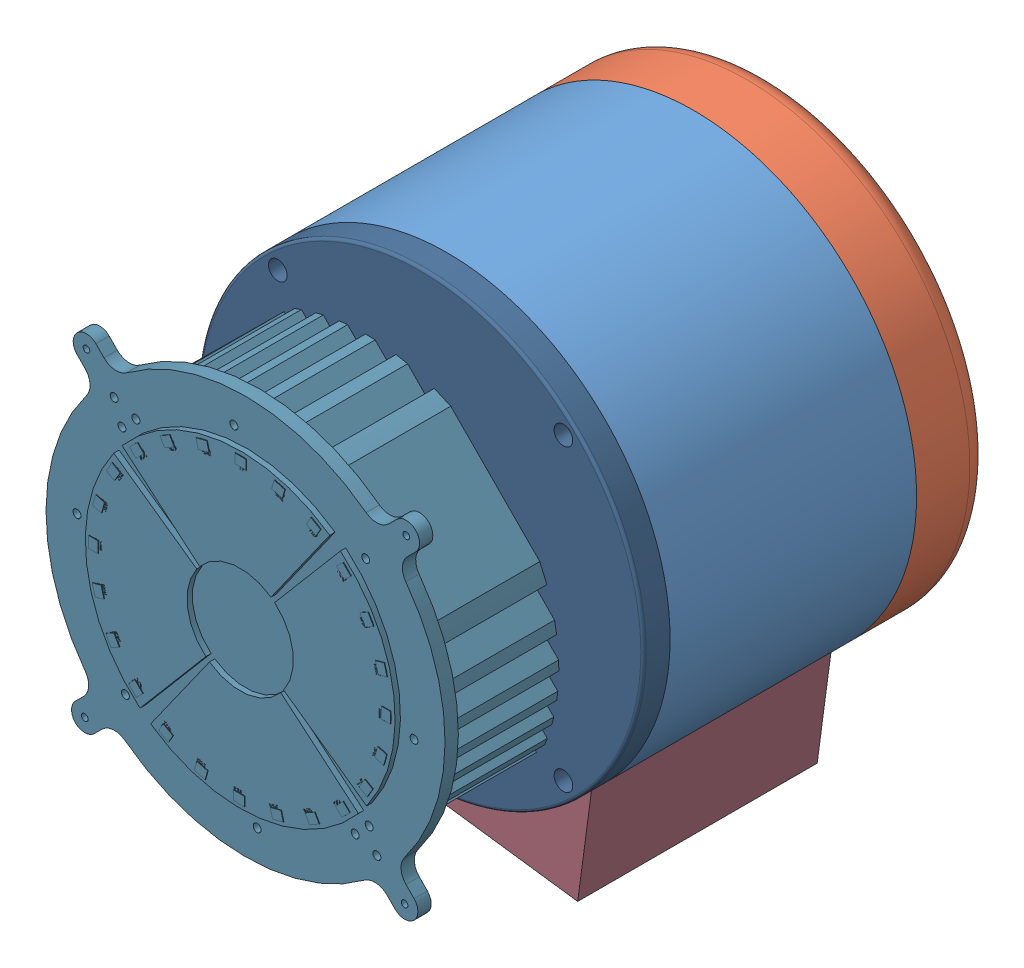
SolidWorks assembly ana montaj, configuration Default. Lengths in mm.
Overall size (509.11 509.11 476.35).
55 component instances, 14 part files, 25 mates.
Components (placement in the parent):
- govde-1: govde [Default] at (48.4605 252.1814 189.017) size (335 335 185.3)
- on kapak-1: on kapak [Default] at (48.4605 252.1814 199.017) x (-0.046825 -0.998903 0) z (0 0 -1) size (335 335 65.53)
- 6212 rulman-1: 6212 rulman [Default] at (48.4605 252.1814 171.017) x (0.999853 -0.01716 0) z (0 0 1) size (110 110 22)
- 6212 rulman-2: 6212 rulman [Default] at (48.4605 252.1814 149.017) x (0.995072 -0.099154 0) z (0 0 1) size (110 110 22)
- mıl-1: mıl [Default] at (48.4605 252.1814 74.017) x (0 0 -1) z (0.969205 -0.246255 0) size (328 80 80)
- toz kecesı-1: toz kecesı [Default] at (48.4605 252.1814 149.017) x (0 0 1) z (-0.923728 -0.383049 0) size (31.43 120 120)
- ROTOR MONTAJI-1: ROTOR MONTAJI [Default] at (-54.9975 347.7347 159.2712) x (-0.212044 -0.97726 0) z (0 0 1) size (204.45 204.45 100)
  - rotor1-1: rotor1 [Varsayılan] at (71.4427 121.3669 64.7458) size (192 192 50)
  - rotor2-1: rotor2 [Varsayılan] at (71.4427 121.3669 164.7458) x (-1 0 0) z (0 0 -1) size (192 192 50)
  - magnet-1: magnet [Varsayılan] at (71.4427 121.3669 64.7458) x (0.951057 0.309017 0) z (0 0 1) size (25.12 8.28 50)
  - magnet-2: magnet [Varsayılan] at (71.4427 121.3669 64.7458) size (25.12 8.28 50)
  - magnet-3: magnet [Varsayılan] at (71.4427 121.3669 64.7458) x (0.951057 -0.309017 0) z (0 0 1) size (25.12 8.28 50)
  - magnet-4: magnet [Varsayılan] at (71.4427 121.3669 64.7458) x (0.809017 -0.587785 0) z (0 0 1) size (25.12 8.28 50)
  - magnet-5: magnet [Varsayılan] at (71.4427 121.3669 64.7458) x (0.587785 -0.809017 0) z (0 0 1) size (25.12 8.28 50)
  - magnet-6: magnet [Varsayılan] at (71.4427 121.3669 64.7458) x (0.309017 -0.951057 0) z (0 0 1) size (25.12 8.28 50)
  - magnet-7: magnet [Varsayılan] at (71.4427 121.3669 64.7458) x (0 -1 0) z (0 0 1) size (25.12 8.28 50)
  - magnet-8: magnet [Varsayılan] at (71.4427 121.3669 64.7458) x (-0.309017 -0.951057 0) z (0 0 1) size (25.12 8.28 50)
  - magnet-9: magnet [Varsayılan] at (71.4427 121.3669 64.7458) x (-0.587785 -0.809017 0) z (0 0 1) size (25.12 8.28 50)
  - magnet-10: magnet [Varsayılan] at (71.4427 121.3669 64.7458) x (-0.809017 -0.587785 0) z (0 0 1) size (25.12 8.28 50)
  - magnet-11: magnet [Varsayılan] at (71.4427 121.3669 64.7458) x (-0.951057 -0.309017 0) z (0 0 1) size (25.12 8.28 50)
  - magnet-12: magnet [Varsayılan] at (71.4427 121.3669 64.7458) x (-1 0 0) z (0 0 1) size (25.12 8.28 50)
  - magnet-13: magnet [Varsayılan] at (71.4427 121.3669 64.7458) x (-0.951057 0.309017 0) z (0 0 1) size (25.12 8.28 50)
  - magnet-14: magnet [Varsayılan] at (71.4427 121.3669 64.7458) x (-0.809017 0.587785 0) z (0 0 1) size (25.12 8.28 50)
  - magnet-15: magnet [Varsayılan] at (71.4427 121.3669 64.7458) x (-0.587785 0.809017 0) z (0 0 1) size (25.12 8.28 50)
  - magnet-16: magnet [Varsayılan] at (71.4427 121.3669 64.7458) x (-0.309017 0.951057 0) z (0 0 1) size (25.12 8.28 50)
  - magnet-17: magnet [Varsayılan] at (71.4427 121.3669 64.7458) x (0 1 0) z (0 0 1) size (25.12 8.28 50)
  - magnet-18: magnet [Varsayılan] at (71.4427 121.3669 64.7458) x (0.309017 0.951057 0) z (0 0 1) size (25.12 8.28 50)
  - magnet-19: magnet [Varsayılan] at (71.4427 121.3669 64.7458) x (0.587785 0.809017 0) z (0 0 1) size (25.12 8.28 50)
  - magnet-20: magnet [Varsayılan] at (71.4427 121.3669 64.7458) x (0.809017 0.587785 0) z (0 0 1) size (25.12 8.28 50)
  - magnet-21: magnet [Varsayılan] at (71.4427 121.3669 14.7458) x (0.951057 0.309017 0) z (0 0 1) size (25.12 8.28 50)
  - magnet-22: magnet [Varsayılan] at (71.4427 121.3669 14.7458) size (25.12 8.28 50)
  - magnet-23: magnet [Varsayılan] at (71.4427 121.3669 14.7458) x (0.951057 -0.309017 0) z (0 0 1) size (25.12 8.28 50)
  - magnet-24: magnet [Varsayılan] at (71.4427 121.3669 14.7458) x (0.809017 -0.587785 0) z (0 0 1) size (25.12 8.28 50)
  - magnet-25: magnet [Varsayılan] at (71.4427 121.3669 14.7458) x (0.587785 -0.809017 0) z (0 0 1) size (25.12 8.28 50)
  - magnet-26: magnet [Varsayılan] at (71.4427 121.3669 14.7458) x (0.309017 -0.951057 0) z (0 0 1) size (25.12 8.28 50)
  - magnet-27: magnet [Varsayılan] at (71.4427 121.3669 14.7458) x (0 -1 0) z (0 0 1) size (25.12 8.28 50)
  - magnet-28: magnet [Varsayılan] at (71.4427 121.3669 14.7458) x (-0.309017 -0.951057 0) z (0 0 1) size (25.12 8.28 50)
  - magnet-29: magnet [Varsayılan] at (71.4427 121.3669 14.7458) x (-0.587785 -0.809017 0) z (0 0 1) size (25.12 8.28 50)
  - magnet-30: magnet [Varsayılan] at (71.4427 121.3669 14.7458) x (-0.809017 -0.587785 0) z (0 0 1) size (25.12 8.28 50)
  - magnet-31: magnet [Varsayılan] at (71.4427 121.3669 14.7458) x (-0.951057 -0.309017 0) z (0 0 1) size (25.12 8.28 50)
  - magnet-32: magnet [Varsayılan] at (71.4427 121.3669 14.7458) x (-1 0 0) z (0 0 1) size (25.12 8.28 50)
  - magnet-33: magnet [Varsayılan] at (71.4427 121.3669 14.7458) x (-0.951057 0.309017 0) z (0 0 1) size (25.12 8.28 50)
  - magnet-34: magnet [Varsayılan] at (71.4427 121.3669 14.7458) x (-0.809017 0.587785 0) z (0 0 1) size (25.12 8.28 50)
  - magnet-35: magnet [Varsayılan] at (71.4427 121.3669 14.7458) x (-0.587785 0.809017 0) z (0 0 1) size (25.12 8.28 50)
  - magnet-36: magnet [Varsayılan] at (71.4427 121.3669 14.7458) x (-0.309017 0.951057 0) z (0 0 1) size (25.12 8.28 50)
  - magnet-37: magnet [Varsayılan] at (71.4427 121.3669 14.7458) x (0 1 0) z (0 0 1) size (25.12 8.28 50)
  - magnet-38: magnet [Varsayılan] at (71.4427 121.3669 14.7458) x (0.309017 0.951057 0) z (0 0 1) size (25.12 8.28 50)
  - magnet-39: magnet [Varsayılan] at (71.4427 121.3669 14.7458) x (0.587785 0.809017 0) z (0 0 1) size (25.12 8.28 50)
  - magnet-40: magnet [Varsayılan] at (71.4427 121.3669 14.7458) x (0.809017 0.587785 0) z (0 0 1) size (25.12 8.28 50)
- stator-1: stator [Varsayılan] at (48.4605 252.1814 224.017) x (0.971789 0.235853 0) z (0 0 1) size (300 300 100)
- arka kapak-1: arka kapak [Default] at (48.4605 252.1814 349.017) x (0 0 1) z (-1 0 0) size (45.3 335 335)
- 6205 rulman-1: 6205 rulman [Default] at (48.4605 252.1814 372.317) x (-0.923728 -0.383049 0) z (0 0 -1) size (62 62 16)
- balans-1: balans [Default] at (48.4605 252.1814 299.017) x (0.633957 -0.773369 0) z (0 0 1) size (70 70 20)
- ayak-1: ayak [Default] at (48.4605 252.1814 189.017) x (0.991146 -0.132778 0) z (0 0 1) size (240 80 180)
- Heatsink_v5-2: Heatsink_v5 [Default] at (48.4605 252.1814 525.9201) x (-0.710787 -0.703407 0) z (-0.703407 0.710787 0) size (360 94.45 360)
Mates (geometry in assembly coordinates):
- Eş Merkezli1: concentric anti-aligned: cylinder of govde-1 through (48.4605 252.1814 374.317) axis (0 0 -1) radius 148; cylinder of on kapak-1 through (48.4605 252.1814 -541.983) axis (0 0 1) radius 55
- Çakışık1: coincident anti-aligned: plane of govde-1 through (48.4605 252.1814 189.017) normal (0 0 -1); plane of on kapak-1 through (48.4605 252.1814 189.017) normal (0 0 1)
- Eş Merkezli2: concentric aligned: cylinder of 6212 rulman-1 through (48.4605 252.1814 193.017) axis (0 0 -1) radius 30; cylinder of 6212 rulman-2 through (48.4605 252.1814 171.017) axis (0 0 -1) radius 30
- Çakışık2: coincident anti-aligned: plane of 6212 rulman-1 through (48.4605 252.1814 171.017) normal (0 0 -1); plane of 6212 rulman-2 through (48.4605 252.1814 171.017) normal (0 0 1)
- Eş Merkezli3: concentric anti-aligned: cylinder of on kapak-1 through (48.4605 252.1814 -541.983) axis (0 0 1) radius 55; cylinder of 6212 rulman-2 through (48.4605 252.1814 171.017) axis (0 0 -1) radius 30
- Uzaklık1: distance = 6 mm aligned: plane of 6212 rulman-1 through (48.4605 252.1814 193.017) normal (0 0 1); plane of on kapak-1 through (48.4605 252.1814 199.017) normal (0 0 1)
- Eş Merkezli4: concentric aligned: cylinder of on kapak-1 through (48.4605 252.1814 -16.5465) axis (0 0 1) radius 38.5; cylinder of mıl-1 through (48.4605 252.1814 382.017) axis (0 0 1) radius 25
- Çakışık5: coincident anti-aligned: plane of 6212 rulman-1 through (48.4605 252.1814 193.017) normal (0 0 1); plane of mıl-1 through (55.8482 281.2576 193.017) normal (0 0 -1)
- Eş Merkezli5: concentric aligned: cylinder of mıl-1 through (48.4605 252.1814 382.017) axis (0 0 1) radius 28; cylinder of toz kecesı-1 through (48.4605 252.1814 149.017) axis (0 0 1) radius 60
- Teğet1: tangent: torus of 6212 rulman-2; plane of toz kecesı-1 through (36.969 279.8933 149.017) normal (0 0 1)
- Eş Merkezli6: concentric anti-aligned: cylinder of mıl-1 through (48.4605 252.1814 382.017) axis (0 0 1) radius 25; cylinder of ROTOR MONTAJI-1/rotor2-1 through (48.4605 252.1814 564.4333) axis (0 0 -1) radius 25
- Çakışık8: coincident anti-aligned: plane of mıl-1 through (58.3107 290.9496 249.017) normal (0 0 1); plane of ROTOR MONTAJI-1/rotor2-1 through (48.4605 252.1814 249.017) normal (0 0 -1)
- Eş Merkezli7: concentric aligned: cylinder of govde-1 through (-58.8894 364.6814 204.017) axis (0 0 -1) radius 3.4; cylinder of on kapak-1 through (-58.8894 364.6814 200.3307) axis (0 0 -1) radius 4
- Eş Merkezli8: concentric: cylinder of govde-1 through (48.4605 252.1814 374.317) axis (0 0 -1) radius 148; cylinder of stator-1 through (48.4605 252.1814 -194.5902) axis (0 0 1) radius 148
- Çakışık9: coincident anti-aligned: plane of govde-1 through (48.4605 411.0892 224.017) normal (0 0 1); plane of stator-1 through (48.4605 252.1814 224.017) normal (0 0 -1)
- Eş Merkezli9: concentric anti-aligned: cylinder of arka kapak-1 through (48.4605 252.1814 349.017) axis (0 0 -1) radius 31; cylinder of 6205 rulman-1 through (48.4605 252.1814 356.317) axis (0 0 1) radius 15
- Çakışık10: coincident aligned: plane of arka kapak-1 through (48.4605 284.9314 356.317) normal (0 0 -1); plane of 6205 rulman-1 through (48.4605 252.1814 356.317) normal (0 0 -1)
- Eş Merkezli10: concentric aligned: cylinder of govde-1 through (48.4605 252.1814 374.317) axis (0 0 -1) radius 148; cylinder of arka kapak-1 through (48.4605 252.1814 349.017) axis (0 0 -1) radius 148
- Çakışık11: coincident anti-aligned: plane of govde-1 through (48.4605 252.1814 374.317) normal (0 0 1); plane of arka kapak-1 through (48.4605 419.6814 374.317) normal (0 0 -1)
- Eş Merkezli11: concentric aligned: cylinder of arka kapak-1 through (48.4605 252.1814 349.017) axis (0 0 -1) radius 167.5; cylinder of balans-1 through (48.4605 252.1814 319.017) axis (0 0 -1) radius 25
- Çakışık12: coincident anti-aligned: plane of ROTOR MONTAJI-1/rotor1-1 through (48.4605 252.1814 299.017) normal (0 0 1); plane of balans-1 through (48.4605 252.1814 299.017) normal (0 0 -1)
- Eş Merkezli12: concentric aligned: cylinder of govde-1 through (-58.8894 364.6814 359.317) axis (0 0 1) radius 3.4; cylinder of arka kapak-1 through (-58.8894 364.6814 363.0033) axis (0 0 1) radius 4
- Eş Merkezli13: concentric aligned: cylinder of govde-1 through (48.4605 252.1814 374.317) axis (0 0 -1) radius 167.5; cylinder of ayak-1 through (48.4605 252.1814 369.017) axis (0 0 -1) radius 167.5
- Çakışık13: coincident anti-aligned: circle of govde-1; plane of ayak-1 through (48.4605 252.1814 189.017) normal (0 0 -1)
- Concentric2: concentric aligned: circle of arka kapak-1; circle of Heatsink_v5-2
